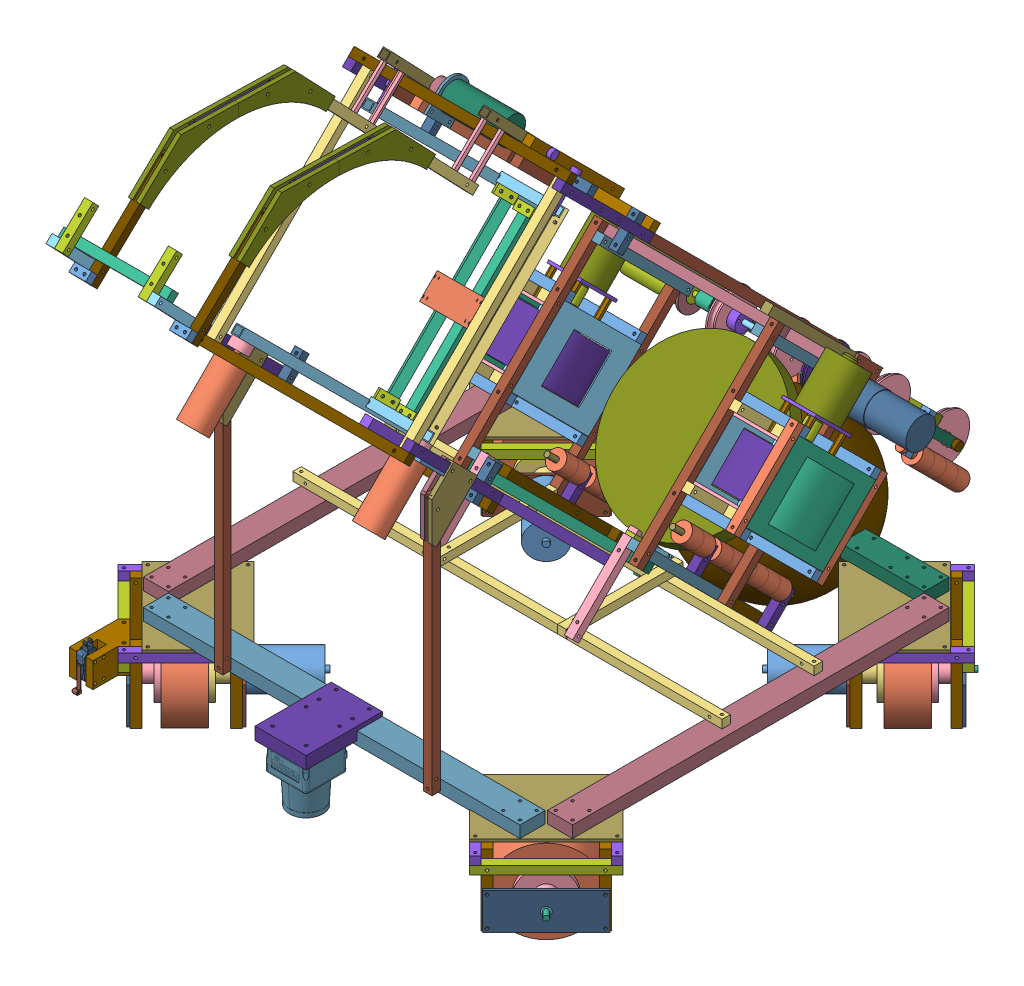
SolidWorks assembly R2, configuration ﾃﾞﾌｫﾙﾄ. Lengths in mm. (continued)
Components (placement in the parent): (continued)
- Copy of Shooter^R2-1: Copy of Shooter^R2 [ﾃﾞﾌｫﾙﾄ] at (-133.6019 -3.3981 619.3345) x (1 0 0) z (0 0.707107 0.707107) size (512.8 347.34 409.41) (virtual, flexible) (continued)
  - Copy of Copy of Copy (2) of Copy of Copy (2) of Copy of Copy (2) of 角材１^Copy of Shooter_R2-3: Copy of Copy of Copy (2) of Copy of Copy (2) of Copy of Copy (2) of 角材１^Copy of Shooter_R2 [ﾃﾞﾌｫﾙﾄ] at (20 10 0) x (0 0 1) z (-1 0 0) size (150 10 10) (virtual)
  - Copy of Copy of Copy (2) of Copy of Copy (2) of Copy of Copy (2) of 角材１^Copy of Shooter_R2-4: Copy of Copy of Copy (2) of Copy of Copy (2) of Copy of Copy (2) of 角材１^Copy of Shooter_R2 [ﾃﾞﾌｫﾙﾄ] at (210 10 0) x (0 0 1) z (-1 0 0) size (150 10 10) (virtual)
  - Part19^Copy of Shooter_R2-1: Part19^Copy of Shooter_R2 [ﾃﾞﾌｫﾙﾄ] at (290 165 10) x (-1 0 0) z (0 0 -1) size (190 190 20) (virtual)
  - Copy (2) of Copy of Copy of Copy of Copy of Copy (2) of Copy of Copy (2) of 角材１^Copy of Shooter_R2-3: Copy (2) of Copy of Copy of Copy of Copy of Copy (2) of Copy of Copy (2) of 角材１^Copy of Shooter_R2 [ﾃﾞﾌｫﾙﾄ] at (180 50 20) x (0 -1 0) z (0 0 1) size (50 10 10) (virtual)
  - Copy of Copy (2) of Copy of Copy of Copy of Copy of Copy (2) of Copy of Copy (2) of 角材１^Copy of Shooter_R2-1: Copy of Copy (2) of Copy of Copy of Copy of Copy of Copy (2) of Copy of Copy (2) of 角材１^Copy of Shooter_R2 [ﾃﾞﾌｫﾙﾄ] at (170 10 140) x (0 0 -1) z (1 0 0) size (250 10 10) (virtual)
  - Part17^Copy of Shooter_R2-2: Part17^Copy of Shooter_R2 [ﾃﾞﾌｫﾙﾄ] at (35 45 -115) x (-0.307741 0.95147 0) z (0 0 1) size (6 6 200) (virtual)
  - Copy (2) of Copy of Copy of Copy of Copy of Copy (2) of Copy of Copy (2) of 角材１^Copy of Shooter_R2-5: Copy (2) of Copy of Copy of Copy of Copy of Copy (2) of Copy of Copy (2) of 角材１^Copy of Shooter_R2 [ﾃﾞﾌｫﾙﾄ] at (30 50 20) x (0 -1 0) z (0 0 1) size (50 10 10) (virtual)
  - Copy of Copy (2) of Copy of Copy of Copy of Copy of Copy (2) of Copy of Copy (2) of 角材１^Copy of Shooter_R2-2: Copy of Copy (2) of Copy of Copy of Copy of Copy of Copy (2) of Copy of Copy (2) of 角材１^Copy of Shooter_R2 [ﾃﾞﾌｫﾙﾄ] at (40 10 140) x (0 0 -1) z (1 0 0) size (250 10 10) (virtual)
  - Copy (3) of Copy of Copy of Copy of Copy of Copy (2) of Copy of Copy (2) of 角材１^Copy of Shooter_R2-1: Copy (3) of Copy of Copy of Copy of Copy of Copy (2) of Copy of Copy (2) of 角材１^Copy of Shooter_R2 [ﾃﾞﾌｫﾙﾄ] at (30 0 -100) size (160 10 10) (virtual)
  - Copy (2) of Copy of Copy of Copy of Copy of Copy (2) of Copy of Copy (2) of 角材１^Copy of Shooter_R2-6: Copy (2) of Copy of Copy of Copy of Copy of Copy (2) of Copy of Copy (2) of 角材１^Copy of Shooter_R2 [ﾃﾞﾌｫﾙﾄ] at (30 50 -110) x (0 -1 0) z (0 0 1) size (50 10 10) (virtual)
  - Copy (2) of Copy of Copy of Copy of Copy of Copy (2) of Copy of Copy (2) of 角材１^Copy of Shooter_R2-7: Copy (2) of Copy of Copy of Copy of Copy of Copy (2) of Copy of Copy (2) of 角材１^Copy of Shooter_R2 [ﾃﾞﾌｫﾙﾄ] at (180 50 -110) x (0 -1 0) z (0 0 1) size (50 10 10) (virtual)
  - Part20^Copy of Shooter_R2-1: Part20^Copy of Shooter_R2 [ﾃﾞﾌｫﾙﾄ] at (185 45 0.2) x (0 1 0) z (0 0 -1) size (21 21 19.8) (virtual)
  - Part20^Copy of Shooter_R2-2: Part20^Copy of Shooter_R2 [ﾃﾞﾌｫﾙﾄ] at (185 45 20) x (0 1 0) z (0 0 -1) size (21 21 19.8) (virtual)
  - Part20^Copy of Shooter_R2-3: Part20^Copy of Shooter_R2 [ﾃﾞﾌｫﾙﾄ] at (185 45 -79) x (0 1 0) z (0 0 -1) size (21 21 19.8) (virtual)
  - Part20^Copy of Shooter_R2-4: Part20^Copy of Shooter_R2 [ﾃﾞﾌｫﾙﾄ] at (185 45 -19.6) x (0 1 0) z (0 0 -1) size (21 21 19.8) (virtual)
  - Part20^Copy of Shooter_R2-5: Part20^Copy of Shooter_R2 [ﾃﾞﾌｫﾙﾄ] at (185 45 -59.2) x (0 1 0) z (0 0 -1) size (21 21 19.8) (virtual)
  - Part20^Copy of Shooter_R2-6: Part20^Copy of Shooter_R2 [ﾃﾞﾌｫﾙﾄ] at (185 45 -39.4) x (0.985931 0.167151 0) z (0 0 -1) size (21 21 19.8) (virtual)
  - Part20^Copy of Shooter_R2-7: Part20^Copy of Shooter_R2 [ﾃﾞﾌｫﾙﾄ] at (35 45 -19.6) x (0 1 0) z (0 0 -1) size (21 21 19.8) (virtual)
  - Part20^Copy of Shooter_R2-8: Part20^Copy of Shooter_R2 [ﾃﾞﾌｫﾙﾄ] at (35 45 20) x (0 1 0) z (0 0 -1) size (21 21 19.8) (virtual)
  - Part20^Copy of Shooter_R2-9: Part20^Copy of Shooter_R2 [ﾃﾞﾌｫﾙﾄ] at (35 45 -39.4) x (0 1 0) z (0 0 -1) size (21 21 19.8) (virtual)
  - Part20^Copy of Shooter_R2-10: Part20^Copy of Shooter_R2 [ﾃﾞﾌｫﾙﾄ] at (35 45 0.2) x (0 1 0) z (0 0 -1) size (21 21 19.8) (virtual)
  - Part20^Copy of Shooter_R2-11: Part20^Copy of Shooter_R2 [ﾃﾞﾌｫﾙﾄ] at (35 45 -59.2) x (0.234145 0.972202 0) z (0 0 -1) size (21 21 19.8) (virtual)
  - Part20^Copy of Shooter_R2-12: Part20^Copy of Shooter_R2 [ﾃﾞﾌｫﾙﾄ] at (35 45 -79) x (0 1 0) z (0 0 -1) size (21 21 19.8) (virtual)
  - Part20^Copy of Shooter_R2-21: Part20^Copy of Shooter_R2 [ﾃﾞﾌｫﾙﾄ] at (35 45 69.6) x (0 1 0) z (0 0 -1) size (21 21 19.8) (virtual)
  - Part20^Copy of Shooter_R2-22: Part20^Copy of Shooter_R2 [ﾃﾞﾌｫﾙﾄ] at (35 45 49.8) x (0 1 0) z (0 0 -1) size (21 21 19.8) (virtual)
  - Part20^Copy of Shooter_R2-23: Part20^Copy of Shooter_R2 [ﾃﾞﾌｫﾙﾄ] at (185 45 69.6) x (0.413014 0.910725 0) z (0 0 -1) size (21 21 19.8) (virtual)
  - Part20^Copy of Shooter_R2-24: Part20^Copy of Shooter_R2 [ﾃﾞﾌｫﾙﾄ] at (185 45 49.8) x (-0.320274 0.947325 0) z (0 0 -1) size (21 21 19.8) (virtual)
  - Copy of Copy of Copy of Copy (2) of Copy of Copy (2) of Copy of Copy (2) of 角材１^Copy of Shooter_R2-1: Copy of Copy of Copy of Copy (2) of Copy of Copy (2) of Copy of Copy (2) of 角材１^Copy of Shooter_R2 [ﾃﾞﾌｫﾙﾄ] at (190 16.9239 46.0051) x (0 -0.707107 0.707107) z (-1 0 0) size (140 10 10) (virtual)
  - Copy of Copy of Copy of Copy (2) of Copy of Copy (2) of Copy of Copy (2) of 角材１^Copy of Shooter_R2-2: Copy of Copy of Copy of Copy (2) of Copy of Copy (2) of Copy of Copy (2) of 角材１^Copy of Shooter_R2 [ﾃﾞﾌｫﾙﾄ] at (40 16.9239 46.0051) x (0 -0.707107 0.707107) z (-1 0 0) size (140 10 10) (virtual)
  - Copy (2) of Copy of Copy of Copy of Copy (2) of Copy of Copy (2) of 角材１^Copy of Shooter_R2-1: Copy (2) of Copy of Copy of Copy of Copy (2) of Copy of Copy (2) of 角材１^Copy of Shooter_R2 [ﾃﾞﾌｫﾙﾄ] at (190 20 150) x (0 -1 0) z (1 0 0) size (100 10 10) (virtual)
  - Copy (2) of Copy of Copy of Copy of Copy (2) of Copy of Copy (2) of 角材１^Copy of Shooter_R2-2: Copy (2) of Copy of Copy of Copy of Copy (2) of Copy of Copy (2) of 角材１^Copy of Shooter_R2 [ﾃﾞﾌｫﾙﾄ] at (20 20 150) x (0 -1 0) z (1 0 0) size (100 10 10) (virtual)
  - Copy of Part14^Copy of Shooter_R2-1: Copy of Part14^Copy of Shooter_R2 [ﾃﾞﾌｫﾙﾄ] at (45.3993 224.2591 -11.1142) x (0 0.083089 -0.996542) z (0 -0.996542 -0.083089) size (6 150 6) (virtual)
  - Copy of Copy of Copy of Copy (2) of Part36^Copy of Shooter_R2-1: Copy of Copy of Copy of Copy (2) of Part36^Copy of Shooter_R2 [ﾃﾞﾌｫﾙﾄ] at (36.0219 185.9032 -80.4602) x (0 0.839725 -0.543011) z (-1 0 0) size (16 16 18) (virtual)
  - Copy (2) of Copy of Part33^Copy of Shooter_R2-2: Copy (2) of Copy of Part33^Copy of Shooter_R2 [ﾃﾞﾌｫﾙﾄ] at (-597.1629 304.0265 -20) x (1 0 0) z (0 0 -1) size (90 32 32) (virtual)
  - Copy (2) of Copy (2) of Part36^Copy of Shooter_R2-2: Copy (2) of Copy (2) of Part36^Copy of Shooter_R2 [ﾃﾞﾌｫﾙﾄ] at (151 153.9641 -31.7433) x (0 -0.163101 0.986609) z (1 0 0) size (22 22 10) (virtual)
  - Copy of Copy of Part36^Copy of Shooter_R2-1: Copy of Copy of Part36^Copy of Shooter_R2 [ﾃﾞﾌｫﾙﾄ] at (179.9858 153.1375 -24.4469) x (0 -0.061762 0.998091) z (1 0 0) size (22 22 10) (virtual)
  - Part22^Copy of Shooter_R2-1: Part22^Copy of Shooter_R2 [ﾃﾞﾌｫﾙﾄ] at (285 218 -20) x (0 0 1) z (0 -1 0) size (37 103 37) (virtual)
  - Part23^Copy of Shooter_R2-1: Part23^Copy of Shooter_R2 [ﾃﾞﾌｫﾙﾄ] at (203 240 -40) x (0 0 1) z (-1 0 0) size (40 52 3) (virtual)
  - Copy of Copy of Copy (2) of Copy of Copy of Copy of Copy of Copy (2) of Copy of Copy (2) of 角材１^Copy of Shooter_R2-1: Copy of Copy of Copy (2) of Copy of Copy of Copy of Copy of Copy (2) of Copy of Copy (2) of 角材１^Copy of Shooter_R2 [ﾃﾞﾌｫﾙﾄ] at (190 240 140) x (0 0 -1) z (1 0 0) size (180 10 10) (virtual)
  - Copy of Copy of Copy (2) of Copy of Copy of Copy of Copy of Copy (2) of Copy of Copy (2) of 角材１^Copy of Shooter_R2-2: Copy of Copy of Copy (2) of Copy of Copy of Copy of Copy of Copy (2) of Copy of Copy (2) of 角材１^Copy of Shooter_R2 [ﾃﾞﾌｫﾙﾄ] at (20 240 140) x (0 0 -1) z (1 0 0) size (180 10 10) (virtual)
  - Part24^Copy of Shooter_R2-1: Part24^Copy of Shooter_R2 [ﾃﾞﾌｫﾙﾄ] at (7 250 -40) x (0 0 1) z (1 0 0) size (40 45 3) (virtual)
  - Copy (4) of Copy of Copy of Copy of Copy of Copy (2) of Copy of Copy (2) of 角材１^Copy of Shooter_R2-2: Copy (4) of Copy of Copy of Copy of Copy of Copy (2) of Copy of Copy (2) of 角材１^Copy of Shooter_R2 [ﾃﾞﾌｫﾙﾄ] at (0 0 10) size (220 10 10) (virtual)
  - Copy (2) of Copy of Copy of Copy of Copy of Copy of Copy of Copy of Copy (2) of Copy of Copy (9) of Copy (2) of 角材１^Copy of Shooter_R2-3: Copy (2) of Copy of Copy of Copy of Copy of Copy of Copy of Copy of Copy (2) of Copy of Copy (9) of Copy (2) of 角材１^Copy of Shooter_R2 [ﾃﾞﾌｫﾙﾄ] at (50 230 -5) x (0 0 -1) z (-1 0 0) size (220 10 10) (virtual)
  - Copy (2) of Copy of Copy of Copy of Copy of Copy of Copy of Copy of Copy (2) of Copy of Copy (9) of Copy (2) of 角材１^Copy of Shooter_R2-4: Copy (2) of Copy of Copy of Copy of Copy of Copy of Copy of Copy of Copy (2) of Copy of Copy (9) of Copy (2) of 角材１^Copy of Shooter_R2 [ﾃﾞﾌｫﾙﾄ] at (180 230 -5) x (0 0 -1) z (-1 0 0) size (220 10 10) (virtual)
  - Copy of Copy of Copy of Copy (2) of Copy of Copy (2) of 角材１^Copy of Shooter_R2-1: Copy of Copy of Copy of Copy (2) of Copy of Copy (2) of 角材１^Copy of Shooter_R2 [ﾃﾞﾌｫﾙﾄ] at (190 240 -170) x (-1 0 0) z (0 0 1) size (160 10 10) (virtual)
  - Copy of Part25^Copy of Shooter_R2-7: Copy of Part25^Copy of Shooter_R2 [ﾃﾞﾌｫﾙﾄ] at (169 225 -20) x (1 0 0) z (0 0.163101 -0.986609) size (8 56 56) (virtual)
  - Copy (2) of Copy (2) of Part36^Copy of Shooter_R2-3: Copy (2) of Copy (2) of Part36^Copy of Shooter_R2 [ﾃﾞﾌｫﾙﾄ] at (69 295.1733 -3.8846) x (0 -0.223824 0.974629) z (-1 0 0) size (22 22 10) (virtual)
  - Part26^Copy of Shooter_R2-3: Part26^Copy of Shooter_R2 [ﾃﾞﾌｫﾙﾄ] at (185 225 -220) x (-1 0 0) z (0 0.743251 -0.669013) size (35 10 10) (virtual)
  - Part26^Copy of Shooter_R2-4: Part26^Copy of Shooter_R2 [ﾃﾞﾌｫﾙﾄ] at (35 225 -220) x (1 0 0) z (0 -0.001736 -0.999998) size (35 10 10) (virtual)
  - Part26^Copy of Shooter_R2-5: Part26^Copy of Shooter_R2 [ﾃﾞﾌｫﾙﾄ] at (185 225 -120) x (-1 0 0) z (0 -0.001736 -0.999998) size (35 10 10) (virtual)
  - Part26^Copy of Shooter_R2-6: Part26^Copy of Shooter_R2 [ﾃﾞﾌｫﾙﾄ] at (35 225 -120) x (1 0 0) z (0 -0.001736 -0.999998) size (35 10 10) (virtual)
  - Copy (3) of Copy of Copy of Copy of Copy (2) of Copy of Copy (2) of 角材１^Copy of Shooter_R2-1: Copy (3) of Copy of Copy of Copy of Copy (2) of Copy of Copy (2) of 角材１^Copy of Shooter_R2 [ﾃﾞﾌｫﾙﾄ] at (190 195 -160) x (0 1 0) z (0 0 1) size (45 10 10) (virtual)
  - Copy (3) of Copy of Copy of Copy of Copy (2) of Copy of Copy (2) of 角材１^Copy of Shooter_R2-2: Copy (3) of Copy of Copy of Copy of Copy (2) of Copy of Copy (2) of 角材１^Copy of Shooter_R2 [ﾃﾞﾌｫﾙﾄ] at (40 195 -160) x (0 1 0) z (0 0 1) size (45 10 10) (virtual)
  - Part20^Copy of Shooter_R2-25: Part20^Copy of Shooter_R2 [ﾃﾞﾌｫﾙﾄ] at (185 200 -184.8) x (0.035115 -0.999383 0) z (0 0 1) size (21 21 19.8) (virtual)
  - Copy of Part26^Copy of Shooter_R2-1: Copy of Part26^Copy of Shooter_R2 [ﾃﾞﾌｫﾙﾄ] at (185 200 -145) x (0 0 -1) z (-0.990327 0.138756 0) size (105 10 10) (virtual)
  - Part20^Copy of Shooter_R2-26: Part20^Copy of Shooter_R2 [ﾃﾞﾌｫﾙﾄ] at (185 200 -204.6) x (-0.121292 -0.992617 0) z (0 0 1) size (21 21 19.8) (virtual)
  - Part20^Copy of Shooter_R2-27: Part20^Copy of Shooter_R2 [ﾃﾞﾌｫﾙﾄ] at (185 200 -224.4) x (0.035115 -0.999383 0) z (0 0 1) size (21 21 19.8) (virtual)
  - Part20^Copy of Shooter_R2-28: Part20^Copy of Shooter_R2 [ﾃﾞﾌｫﾙﾄ] at (185 200 -244.2) x (0.035115 -0.999383 0) z (0 0 1) size (21 21 19.8) (virtual)
  - Part20^Copy of Shooter_R2-29: Part20^Copy of Shooter_R2 [ﾃﾞﾌｫﾙﾄ] at (35 200 -184.8) x (0.035115 -0.999383 0) z (0 0 1) size (21 21 19.8) (virtual)
  - Part20^Copy of Shooter_R2-30: Part20^Copy of Shooter_R2 [ﾃﾞﾌｫﾙﾄ] at (35 200 -204.6) x (-0.121292 -0.992617 0) z (0 0 1) size (21 21 19.8) (virtual)
  - Copy of Part26^Copy of Shooter_R2-2: Copy of Part26^Copy of Shooter_R2 [ﾃﾞﾌｫﾙﾄ] at (35 200 -145) x (0 0 -1) z (-0.990327 0.138756 0) size (105 10 10) (virtual)
  - Part20^Copy of Shooter_R2-31: Part20^Copy of Shooter_R2 [ﾃﾞﾌｫﾙﾄ] at (35 200 -224.4) x (0.035115 -0.999383 0) z (0 0 1) size (21 21 19.8) (virtual)
  - Part20^Copy of Shooter_R2-32: Part20^Copy of Shooter_R2 [ﾃﾞﾌｫﾙﾄ] at (35 200 -244.2) x (0.035115 -0.999383 0) z (0 0 1) size (21 21 19.8) (virtual)
  - Copy of Copy (4) of Copy of Copy of Copy of Copy (2) of Copy of Copy (2) of 角材１^Copy of Shooter_R2-1: Copy of Copy (4) of Copy of Copy of Copy of Copy (2) of Copy of Copy (2) of 角材１^Copy of Shooter_R2 [ﾃﾞﾌｫﾙﾄ] at (366.4 -75 137.9289) x (-1 0 0) z (0 -0.707107 -0.707107) size (512.8 10 10) (virtual)
  - Copy of Copy (4) of Copy of Copy of Copy of Copy (2) of Copy of Copy (2) of 角材１^Copy of Shooter_R2-2: Copy of Copy (4) of Copy of Copy of Copy of Copy (2) of Copy of Copy (2) of 角材１^Copy of Shooter_R2 [ﾃﾞﾌｫﾙﾄ] at (366.4 2.7817 60.1472) x (-1 0 0) z (0 -0.707107 -0.707107) size (512.8 10 10) (virtual)
  - Part25^Copy of Shooter_R2-5: Part25^Copy of Shooter_R2 [ﾃﾞﾌｫﾙﾄ] at (169 225 -120) x (1 0 0) z (0 -0.163101 0.986609) size (8 56 56) (virtual)
  - Part25^Copy of Shooter_R2-6: Part25^Copy of Shooter_R2 [ﾃﾞﾌｫﾙﾄ] at (169 225 -220) x (1 0 0) z (0 0.431687 0.902023) size (8 56 56) (virtual)
  - Part25^Copy of Shooter_R2-7: Part25^Copy of Shooter_R2 [ﾃﾞﾌｫﾙﾄ] at (51 225 -120) x (-1 0 0) z (0 -0.974129 -0.225994) size (8 56 56) (virtual)
  - Part25^Copy of Shooter_R2-8: Part25^Copy of Shooter_R2 [ﾃﾞﾌｫﾙﾄ] at (51 225 -220) x (-1 0 0) z (0 -0.974129 -0.225994) size (8 56 56) (virtual)
  - Part27^Copy of Shooter_R2-1: Part27^Copy of Shooter_R2 [ﾃﾞﾌｫﾙﾄ] at (0 155.2 149.8) x (0 0 -1) z (1 0 0) size (129.6 89.6 10) (virtual)
  - Copy of Part27^Copy of Shooter_R2-1: Copy of Part27^Copy of Shooter_R2 [ﾃﾞﾌｫﾙﾄ] at (280 155.2 149.8) x (0 0 -1) z (1 0 0) size (129.6 89.6 26) (virtual)
  - Part27^Copy of Shooter_R2-3: Part27^Copy of Shooter_R2 [ﾃﾞﾌｫﾙﾄ] at (220 154.8 -0.2) x (0 0 1) z (-1 0 0) size (129.6 89.6 10) (virtual)
  - Copy of Part27^Copy of Shooter_R2-2: Copy of Part27^Copy of Shooter_R2 [ﾃﾞﾌｫﾙﾄ] at (-60 155.2 -0.2) x (0 0 1) z (-1 0 0) size (129.6 89.6 26) (virtual)
  - Copy of Copy of Part9^Copy of Shooter_R2-1: Copy of Copy of Part9^Copy of Shooter_R2 [ﾃﾞﾌｫﾙﾄ] at (115.15 -0.5946 0.9681) x (0 0 1) z (-1 0 0) size (50 10.5 10) (virtual)
  - Copy of Copy of Part8^Copy of Shooter_R2-1: Copy of Copy of Part8^Copy of Shooter_R2 [ﾃﾞﾌｫﾙﾄ] at (125.15 -0.5946 0.9681) x (0 0 1) z (-1 0 0) size (42.8 26.9 30.3) (virtual)
  - Copy of Copy of D3V-016-1C23^Copy of Shooter_R2-1: Copy of Copy of D3V-016-1C23^Copy of Shooter_R2 [ﾃﾞﾌｫﾙﾄ] at (105.15 -0.25 2.2) x (-1 0 0) z (0 0 -1) size (10.3 26.4 49.2) (virtual)
    - D3V_016_1C23_BASE^Copy of Copy of D3V-016-1C23_Copy of Shooter_R2-1: D3V_016_1C23_BASE^Copy of Copy of D3V-016-1C23_Copy of Shooter_R2 [ﾃﾞﾌｫﾙﾄ] at origin size (10.3 19.05 37.8) (virtual)
    - D3V_016_1C23_LEVER^Copy of Copy of D3V-016-1C23_Copy of Shooter_R2-1: D3V_016_1C23_LEVER^Copy of Copy of D3V-016-1C23_Copy of Shooter_R2 [ﾃﾞﾌｫﾙﾄ] at (-4.8 14.7 -11.8) x (0 0 -1) z (1 0 0) size (28.3 7.35 7.1) (virtual)
    - D3V_016_1C23_BUTTON^Copy of Copy of D3V-016-1C23_Copy of Shooter_R2-1: D3V_016_1C23_BUTTON^Copy of Copy of D3V-016-1C23_Copy of Shooter_R2 [ﾃﾞﾌｫﾙﾄ] at (-4.85 11.6 2) size (4.3 3.1 2.8) (virtual)
  - Copy of Copy (2) of Copy of Part9^Copy of Shooter_R2-1: Copy of Copy (2) of Copy of Part9^Copy of Shooter_R2 [ﾃﾞﾌｫﾙﾄ] at (104.85 240.3946 -179.0319) x (0 0 1) z (1 0 0) size (100 13.5 10) (virtual)
  - Copy (2) of Copy of Part8^Copy of Shooter_R2-2: Copy (2) of Copy of Part8^Copy of Shooter_R2 [ﾃﾞﾌｫﾙﾄ] at (94.85 240.3946 -179.0319) x (0 0 1) z (1 0 0) size (42.8 26.9 30.3) (virtual)
  - Copy (2) of Copy of D3V-016-1C23^Copy of Shooter_R2-2: Copy (2) of Copy of D3V-016-1C23^Copy of Shooter_R2 [ﾃﾞﾌｫﾙﾄ] at (114.85 240.05 -177.8) x (1 0 0) z (0 0 -1) size (10.3 26.4 49.2) (virtual)
    - D3V_016_1C23_BASE^Copy (2) of Copy of D3V-016-1C23_Copy of Shooter_R2-1: D3V_016_1C23_BASE^Copy (2) of Copy of D3V-016-1C23_Copy of Shooter_R2 [ﾃﾞﾌｫﾙﾄ] at origin size (10.3 19.05 37.8) (virtual)
    - D3V_016_1C23_LEVER^Copy (2) of Copy of D3V-016-1C23_Copy of Shooter_R2-1: D3V_016_1C23_LEVER^Copy (2) of Copy of D3V-016-1C23_Copy of Shooter_R2 [ﾃﾞﾌｫﾙﾄ] at (-4.8 14.7 -11.8) x (0 0 -1) z (1 0 0) size (28.3 7.35 7.1) (virtual)
    - D3V_016_1C23_BUTTON^Copy (2) of Copy of D3V-016-1C23_Copy of Shooter_R2-1: D3V_016_1C23_BUTTON^Copy (2) of Copy of D3V-016-1C23_Copy of Shooter_R2 [ﾃﾞﾌｫﾙﾄ] at (-4.85 11.6 2) size (4.3 3.1 2.8) (virtual)
  - Part25^Copy of Shooter_R2-9: Part25^Copy of Shooter_R2 [ﾃﾞﾌｫﾙﾄ] at (51 225 -20) x (-1 0 0) z (0 -0.974129 -0.225994) size (8 56 56) (virtual)
- Copy of Rail^R2-1: Copy of Rail^R2 [ﾃﾞﾌｫﾙﾄ] at (-153.6019 377.0254 1016.7285) x (1 0 0) z (0 0.707107 0.707107) size (260 373 863.92) (virtual, flexible)
  - Copy of 角材１^Copy of Rail_R2-1: Copy of 角材１^Copy of Rail_R2 [ﾃﾞﾌｫﾙﾄ] at (260 10 -150) x (0 0 1) z (0 -1 0) size (150 10 10) (virtual)
  - Copy of 角材１^Copy of Rail_R2-2: Copy of 角材１^Copy of Rail_R2 [ﾃﾞﾌｫﾙﾄ] at (10 10 -150) x (0 0 1) z (0 -1 0) size (150 10 10) (virtual)
  - Copy of Copy of 角材１^Copy of Rail_R2-1: Copy of Copy of 角材１^Copy of Rail_R2 [ﾃﾞﾌｫﾙﾄ] at (0 0 -10) x (1 0 0) z (0 -1 0) size (260 10 10) (virtual)
  - Copy of Part24^Copy of Rail_R2-1: Copy of Part24^Copy of Rail_R2 [ﾃﾞﾌｫﾙﾄ] at (260 -3 -20) x (0 0 -1) z (0 1 0) size (40 45 3) (virtual)
  - Copy of Copy (2) of Copy of Part33^Copy of Rail_R2-1: Copy of Copy (2) of Copy of Part33^Copy of Rail_R2 [ﾃﾞﾌｫﾙﾄ] at (314.0265 -607.1629 -40) x (0 1 0) z (0 0 1) size (90 32 32) (virtual)
  - Copy of Copy of Copy of 角材１^Copy of Rail_R2-1: Copy of Copy of Copy of 角材１^Copy of Rail_R2 [ﾃﾞﾌｫﾙﾄ] at (240 -10 -10) x (0 1 0) z (0 0 -1) size (284 10 10) (virtual)
  - Copy of Copy of Copy of 角材１^Copy of Rail_R2-2: Copy of Copy of Copy of 角材１^Copy of Rail_R2 [ﾃﾞﾌｫﾙﾄ] at (10 -10 -10) x (0 1 0) z (0 0 -1) size (284 10 10) (virtual)
  - Copy of Copy of Copy of Part36^Copy of Rail_R2-1: Copy of Copy of Copy of Part36^Copy of Rail_R2 [ﾃﾞﾌｫﾙﾄ] at (285.6516 15 -91.1704) x (-0.7107 0 -0.703495) z (0 -1 0) size (22 22 10) (virtual)
  - Copy of Copy (2) of Copy of Copy of Copy of Copy of Copy of Copy of Copy of Copy (2) of Copy of Copy (9) of Copy (2) of 角材１^Copy of Rail_R2-1: Copy of Copy (2) of Copy of Copy of Copy of Copy of Copy of Copy of Copy of Copy (2) of Copy of Copy (9) of Copy (2) of 角材１^Copy of Rail_R2 [ﾃﾞﾌｫﾙﾄ] at (249.178 15 -33.0011) x (-0.7107 0 -0.703495) z (0 1 0) size (300 10 10) (virtual)
  - Copy of Copy of Copy of Copy of 角材１^Copy of Rail_R2-1: Copy of Copy of Copy of Copy of 角材１^Copy of Rail_R2 [ﾃﾞﾌｫﾙﾄ] at (35.9679 15 -244.0495) x (0 1 0) z (0.703495 0 -0.7107) size (230 10 10) (virtual)
  - Copy of Copy of Copy of Copy of Copy of 角材１^Copy of Rail_R2-1: Copy of Copy of Copy of Copy of Copy of 角材１^Copy of Rail_R2 [ﾃﾞﾌｫﾙﾄ] at (36.0399 35 -229.9076) x (0.703495 0 -0.7107) z (0 -1 0) size (20 10 10) (virtual)
  - Copy of Copy of Copy of Copy of Copy of 角材１^Copy of Rail_R2-2: Copy of Copy of Copy of Copy of Copy of 角材１^Copy of Rail_R2 [ﾃﾞﾌｫﾙﾄ] at (36.0399 235 -229.9076) x (0.703495 0 -0.7107) z (0 -1 0) size (20 10 10) (virtual)
  - Copy of Copy (2) of Copy of Copy of Copy of Copy of Copy of Copy of Copy of Copy (2) of Copy of Copy (9) of Copy (2) of 角材１^Copy of Rail_R2-2: Copy of Copy (2) of Copy of Copy of Copy of Copy of Copy of Copy of Copy of Copy (2) of Copy of Copy (9) of Copy (2) of 角材１^Copy of Rail_R2 [ﾃﾞﾌｫﾙﾄ] at (249.178 235 -33.0011) x (-0.7107 0 -0.703495) z (0 1 0) size (300 10 10) (virtual)
  - Copy of Copy of Copy of Copy of Copy of 角材１^Copy of Rail_R2-3: Copy of Copy of Copy of Copy of Copy of 角材１^Copy of Rail_R2 [ﾃﾞﾌｫﾙﾄ] at (29.985 22 -315.0003) x (-1 0 0.000054) z (0 1 0) size (20 10 10) (virtual)
  - Copy of Copy of Copy of Copy of Copy of 角材１^Copy of Rail_R2-4: Copy of Copy of Copy of Copy of Copy of 角材１^Copy of Rail_R2 [ﾃﾞﾌｫﾙﾄ] at (29.985 222 -315.0003) x (-1 0 0.000054) z (0 1 0) size (20 10 10) (virtual)
  - Copy of Copy (2) of Copy of Copy of Copy of Copy of Copy of Copy of Copy of Copy (2) of Copy of Copy (9) of Copy (2) of 角材１^Copy of Rail_R2-3: Copy of Copy (2) of Copy of Copy of Copy of Copy of Copy of Copy of Copy of Copy (2) of Copy of Copy (9) of Copy (2) of 角材１^Copy of Rail_R2 [ﾃﾞﾌｫﾙﾄ] at (20.0008 22 -24.9997) x (-0.000054 0 -1) z (0 -1 0) size (300 10 10) (virtual)
  - Copy of Copy (2) of Copy of Copy of Copy of Copy of Copy of Copy of Copy of Copy (2) of Copy of Copy (9) of Copy (2) of 角材１^Copy of Rail_R2-4: Copy of Copy (2) of Copy of Copy of Copy of Copy of Copy of Copy of Copy of Copy (2) of Copy of Copy (9) of Copy (2) of 角材１^Copy of Rail_R2 [ﾃﾞﾌｫﾙﾄ] at (20.0008 242 -24.9997) x (-0.000054 0 -1) z (0 -1 0) size (300 10 10) (virtual)
  - Copy of Copy of Copy of Copy of 角材１^Copy of Rail_R2-3: Copy of Copy of Copy of Copy of 角材１^Copy of Rail_R2 [ﾃﾞﾌｫﾙﾄ] at (19.9845 242 -324.9997) x (0 -1 0) z (-1 0 0.000054) size (230 10 10) (virtual)
  - Copy of Copy (2) of Copy of Part33^Copy of Rail_R2-2: Copy of Copy (2) of Copy of Part33^Copy of Rail_R2 [ﾃﾞﾌｫﾙﾄ] at (-54.0265 -607.1629 -40) x (0 1 0) z (0 0 -1) size (90 32 32) (virtual)
  - Copy of Part24^Copy of Rail_R2-2: Copy of Part24^Copy of Rail_R2 [ﾃﾞﾌｫﾙﾄ] at (0 -3 -60) x (0 0 1) z (0 1 0) size (40 45 3) (virtual)
  - Copy of Copy of Copy of Part36^Copy of Rail_R2-2: Copy of Copy of Copy of Part36^Copy of Rail_R2 [ﾃﾞﾌｫﾙﾄ] at (-47 12 -39.9961) x (0.000054 0 1) z (0 -1 0) size (22 22 10) (virtual)
  - Copy (2) of Copy (2) of Copy of Copy of Copy of Copy of 角材１^Copy of Rail_R2-1: Copy (2) of Copy (2) of Copy of Copy of Copy of Copy of 角材１^Copy of Rail_R2 [ﾃﾞﾌｫﾙﾄ] at (210 10 -420) x (0 0 1) z (0 -1 0) size (420 10 10) (virtual)
  - Copy of Copy of 角材１^Copy of Rail_R2-3: Copy of Copy of 角材１^Copy of Rail_R2 [ﾃﾞﾌｫﾙﾄ] at (0 0 -150) x (1 0 0) z (0 -1 0) size (260 10 10) (virtual)
  - Copy of 角材１^Copy of Rail_R2-5: Copy of 角材１^Copy of Rail_R2 [ﾃﾞﾌｫﾙﾄ] at (0 254 -150) x (0 0 1) z (0 1 0) size (150 10 10) (virtual)
  - Copy of Copy of 角材１^Copy of Rail_R2-4: Copy of Copy of 角材１^Copy of Rail_R2 [ﾃﾞﾌｫﾙﾄ] at (260 264 -10) x (-1 0 0) z (0 1 0) size (260 10 10) (virtual)
  - Copy of 角材１^Copy of Rail_R2-6: Copy of 角材１^Copy of Rail_R2 [ﾃﾞﾌｫﾙﾄ] at (250 254 -150) x (0 0 1) z (0 1 0) size (150 10 10) (virtual)
  - Copy (2) of Copy of Copy of 角材１^Copy of Rail_R2-1: Copy (2) of Copy of Copy of 角材１^Copy of Rail_R2 [ﾃﾞﾌｫﾙﾄ] at (260 264 -150) x (-1 0 0) z (0 1 0) size (260 10 10) (virtual)
  - Copy (2) of Copy of Copy of Copy of 角材１^Copy of Rail_R2-1: Copy (2) of Copy of Copy of Copy of 角材１^Copy of Rail_R2 [ﾃﾞﾌｫﾙﾄ] at (10 -10 -130) x (0 1 0) z (0 0 -1) size (40 10 10) (virtual)
  - Copy (2) of Copy of Copy of Copy of 角材１^Copy of Rail_R2-2: Copy (2) of Copy of Copy of Copy of 角材１^Copy of Rail_R2 [ﾃﾞﾌｫﾙﾄ] at (240 -10 -130) x (0 1 0) z (0 0 -1) size (40 10 10) (virtual)
  - Copy (2) of Copy of Copy of Copy of 角材１^Copy of Rail_R2-3: Copy (2) of Copy of Copy of Copy of 角材１^Copy of Rail_R2 [ﾃﾞﾌｫﾙﾄ] at (240 234 -130) x (0 1 0) z (0 0 -1) size (40 10 10) (virtual)
  - Copy (2) of Copy of Copy of Copy of 角材１^Copy of Rail_R2-4: Copy (2) of Copy of Copy of Copy of 角材１^Copy of Rail_R2 [ﾃﾞﾌｫﾙﾄ] at (10 234 -130) x (0 1 0) z (0 0 -1) size (40 10 10) (virtual)
  - Copy (2) of Copy of Copy of Copy of Copy of 角材１^Copy of Rail_R2-3: Copy (2) of Copy of Copy of Copy of Copy of 角材１^Copy of Rail_R2 [ﾃﾞﾌｫﾙﾄ] at (60 264 -540) x (0 0 1) z (0 -1 0) size (540 10 10) (virtual)
  - Copy (2) of Copy of Copy of Copy of Copy of 角材１^Copy of Rail_R2-4: Copy (2) of Copy of Copy of Copy of Copy of 角材１^Copy of Rail_R2 [ﾃﾞﾌｫﾙﾄ] at (210 264 -540) x (0 0 1) z (0 -1 0) size (540 10 10) (virtual)
  - Copy of Copy of Copy of Copy of Copy (2) of Copy of Copy of Copy of Copy of Copy of Copy of Copy of Copy (2) of Copy of Copy (9) of Copy (2) of 角材１^Copy of Rail_R2-1: Copy of Copy of Copy of Copy of Copy (2) of Copy of Copy of Copy of Copy of Copy of Copy of Copy of Copy (2) of Copy of Copy (9) of Copy (2) of 角材１^Copy of Rail_R2 [ﾃﾞﾌｫﾙﾄ] at (65 283.6592 -45.1093) x (0 0.022635 0.999744) z (1 0 0) size (100 10 10) (virtual)
  - Copy of Copy of Copy of Copy of Copy of Part36^Copy of Rail_R2-1: Copy of Copy of Copy of Copy of Copy of Part36^Copy of Rail_R2 [ﾃﾞﾌｫﾙﾄ] at (75 350.9816 -31.6297) x (0 -0.022635 -0.999744) z (1 0 0) size (22 22 10) (virtual)
  - Copy of Copy of Copy of Part24^Copy of Rail_R2-1: Copy of Copy of Copy of Part24^Copy of Rail_R2 [ﾃﾞﾌｫﾙﾄ] at (93 254 -50) x (0 0 1) z (-1 0 0) size (40 45 3) (virtual)
  - Copy of Copy of Copy of Copy (2) of Copy of Part33^Copy of Rail_R2-1: Copy of Copy of Copy of Copy (2) of Copy of Part33^Copy of Rail_R2 [ﾃﾞﾌｫﾙﾄ] at (697.1629 199.9735 -30) x (-1 0 0) z (0 0 -1) size (90 32 32) (virtual)
  - Part1^Copy of Rail_R2-1: Part1^Copy of Rail_R2 [ﾃﾞﾌｫﾙﾄ] at (77 64.3851 99.8911) x (0 -0.999744 0.022635) z (-1 0 0) size (58.93 116.67 5) (virtual)
  - Part1^Copy of Rail_R2-2: Part1^Copy of Rail_R2 [ﾃﾞﾌｫﾙﾄ] at (63 64.3851 99.8911) x (0 -0.722931 -0.69092) z (1 0 0) size (58.93 116.67 5) (virtual)
  - Copy (2) of Copy (3) of Copy of Copy of Copy of Copy of 角材１^Copy of Rail_R2-1: Copy (2) of Copy (3) of Copy of Copy of Copy of Copy of 角材１^Copy of Rail_R2 [ﾃﾞﾌｫﾙﾄ] at (75 140.086 241.403) x (0 0.69092 -0.722931) z (0 0.722931 0.69092) size (100 10 10) (virtual)
  - Copy of Copy (3) of Copy of Copy of Copy of Copy of 角材１^Copy of Rail_R2-1: Copy of Copy (3) of Copy of Copy of Copy of Copy of 角材１^Copy of Rail_R2 [ﾃﾞﾌｫﾙﾄ] at (75 -12.1426 254.1628) x (0 0.999744 -0.022635) z (0 0.022635 0.999744) size (130 10 10) (virtual)
  - Part1^Copy of Rail_R2-3: Part1^Copy of Rail_R2 [ﾃﾞﾌｫﾙﾄ] at (63 64.3851 99.8911) x (0 -0.022635 -0.999744) z (1 0 0) size (58.93 116.67 5) (virtual)
  - Part1^Copy of Rail_R2-4: Part1^Copy of Rail_R2 [ﾃﾞﾌｫﾙﾄ] at (77 64.3851 99.8911) x (0 -0.722931 -0.69092) z (-1 0 0) size (58.93 116.67 5) (virtual)
  - Copy of Copy (2) of Copy (3) of Copy of Copy of Copy of Copy of 角材１^Copy of Rail_R2-1: Copy of Copy (2) of Copy (3) of Copy of Copy of Copy of Copy of 角材１^Copy of Rail_R2 [ﾃﾞﾌｫﾙﾄ] at (75 -1.6924 273.9313) x (-1 0 0) z (0 -0.999744 0.022635) size (20 10 10) (virtual)
  - Copy of Copy of Copy of Copy (2) of Copy (3) of Copy of Copy of Copy of Copy of 角材１^Copy of Rail_R2-1: Copy of Copy of Copy of Copy (2) of Copy (3) of Copy of Copy of Copy of Copy of 角材１^Copy of Rail_R2 [ﾃﾞﾌｫﾙﾄ] at (90 254 0) x (0 0 -1) z (0 1 0) size (150 10 10) (virtual)
  - Copy (2) of Copy of Copy (2) of Copy (3) of Copy of Copy of Copy of Copy of 角材１^Copy of Rail_R2-1: Copy (2) of Copy of Copy (2) of Copy (3) of Copy of Copy of Copy of Copy of 角材１^Copy of Rail_R2 [ﾃﾞﾌｫﾙﾄ] at (75 217.9778 146.4264) x (0 -0.022635 -0.999744) z (0 0.999744 -0.022635) size (130 10 10) (virtual)
  - Copy of Copy of Copy of Part14^Copy of Rail_R2-1: Copy of Copy of Copy of Part14^Copy of Rail_R2 [ﾃﾞﾌｫﾙﾄ] at (70 275.133 20.1004) x (0.021304 0.02263 0.999517) z (0 -0.999744 0.022635) size (6.34 5.64 50) (virtual)
  - Copy of Copy of Copy of Part14^Copy of Rail_R2-2: Copy of Copy of Copy of Part14^Copy of Rail_R2 [ﾃﾞﾌｫﾙﾄ] at (70 275.8121 50.0927) x (0.526034 -0.01925 -0.850246) z (0 -0.999744 0.022635) size (6.34 5.64 50) (virtual)
  - Copy (3) of Copy of Copy (2) of Copy (3) of Copy of Copy of Copy of Copy of 角材１^Copy of Rail_R2-1: Copy (3) of Copy of Copy (2) of Copy (3) of Copy of Copy of Copy of Copy of 角材１^Copy of Rail_R2 [ﾃﾞﾌｫﾙﾄ] at (65 9.4367 323.6922) x (0 -0.022635 -0.999744) z (-1 0 0) size (70 10 10) (virtual)
  - Copy of Copy of Copy (3) of Copy of Copy (2) of Copy (3) of Copy of Copy of Copy of Copy of 角材１^Copy of Rail_R2-1: Copy of Copy of Copy (3) of Copy of Copy (2) of Copy (3) of Copy of Copy of Copy of Copy of 角材１^Copy of Rail_R2 [ﾃﾞﾌｫﾙﾄ] at (185 8.984 303.6973) x (-1 0 0) z (0 0.999744 -0.022635) size (130 10 10) (virtual)
  - Copy of Copy (3) of Copy of Copy (2) of Copy (3) of Copy of Copy of Copy of Copy of 角材１^Copy of Rail_R2-2: Copy of Copy (3) of Copy of Copy (2) of Copy (3) of Copy of Copy of Copy of Copy of 角材１^Copy of Rail_R2 [ﾃﾞﾌｫﾙﾄ] at (65 49.4265 322.7868) x (0 -0.999744 0.022635) z (1 0 0) size (50 10 10) (virtual)
  - Copy of Copy (2) of Copy (3) of Copy of Copy of Copy of Copy of 角材１^Copy of Rail_R2-3: Copy of Copy (2) of Copy (3) of Copy of Copy of Copy of Copy of 角材１^Copy of Rail_R2 [ﾃﾞﾌｫﾙﾄ] at (195 -1.6924 273.9313) x (-1 0 0) z (0 -0.999744 0.022635) size (20 10 10) (virtual)
  - Copy (3) of Copy of Copy (2) of Copy (3) of Copy of Copy of Copy of Copy of 角材１^Copy of Rail_R2-3: Copy (3) of Copy of Copy (2) of Copy (3) of Copy of Copy of Copy of Copy of 角材１^Copy of Rail_R2 [ﾃﾞﾌｫﾙﾄ] at (185 9.4367 323.6922) x (0 -0.022635 -0.999744) z (-1 0 0) size (70 10 10) (virtual)
  - Copy of Copy (3) of Copy of Copy (2) of Copy (3) of Copy of Copy of Copy of Copy of 角材１^Copy of Rail_R2-3: Copy of Copy (3) of Copy of Copy (2) of Copy (3) of Copy of Copy of Copy of Copy of 角材１^Copy of Rail_R2 [ﾃﾞﾌｫﾙﾄ] at (165 49.4265 322.7868) x (0 -0.999744 0.022635) z (1 0 0) size (50 10 10) (virtual)
  - Copy of Copy of Copy of Copy of Copy (2) of Copy of Copy of Copy of Copy of Copy of Copy of Copy of Copy (2) of Copy of Copy (9) of Copy (2) of 角材１^Copy of Rail_R2-2: Copy of Copy of Copy of Copy of Copy (2) of Copy of Copy of Copy of Copy of Copy of Copy of Copy of Copy (2) of Copy of Copy (9) of Copy (2) of 角材１^Copy of Rail_R2 [ﾃﾞﾌｫﾙﾄ] at (185 283.6592 -45.1093) x (0 0.022635 0.999744) z (1 0 0) size (100 10 10) (virtual)
  - Copy of Copy of Copy of Part14^Copy of Rail_R2-3: Copy of Copy of Copy of Part14^Copy of Rail_R2 [ﾃﾞﾌｫﾙﾄ] at (190 275.133 20.1004) x (0.526034 -0.01925 -0.850246) z (0 -0.999744 0.022635) size (6.34 5.64 50) (virtual)
  - Copy (2) of Copy of Copy (2) of Copy (3) of Copy of Copy of Copy of Copy of 角材１^Copy of Rail_R2-2: Copy (2) of Copy of Copy (2) of Copy (3) of Copy of Copy of Copy of Copy of 角材１^Copy of Rail_R2 [ﾃﾞﾌｫﾙﾄ] at (195 217.9778 146.4264) x (0 -0.022635 -0.999744) z (0 0.999744 -0.022635) size (130 10 10) (virtual)
  - Copy of Copy of Copy of Part14^Copy of Rail_R2-4: Copy of Copy of Copy of Part14^Copy of Rail_R2 [ﾃﾞﾌｫﾙﾄ] at (190 275.8121 50.0927) x (0.526034 -0.01925 -0.850246) z (0 -0.999744 0.022635) size (6.34 5.64 50) (virtual)
  - Part1^Copy of Rail_R2-6: Part1^Copy of Rail_R2 [ﾃﾞﾌｫﾙﾄ] at (183 64.3851 99.8911) x (0 -0.722931 -0.69092) z (1 0 0) size (58.93 116.67 5) (virtual)
  - Copy (2) of Copy (3) of Copy of Copy of Copy of Copy of 角材１^Copy of Rail_R2-2: Copy (2) of Copy (3) of Copy of Copy of Copy of Copy of 角材１^Copy of Rail_R2 [ﾃﾞﾌｫﾙﾄ] at (195 140.086 241.403) x (0 0.69092 -0.722931) z (0 0.722931 0.69092) size (100 10 10) (virtual)
  - Part1^Copy of Rail_R2-7: Part1^Copy of Rail_R2 [ﾃﾞﾌｫﾙﾄ] at (197 64.3851 99.8911) x (0 -0.999744 0.022635) z (-1 0 0) size (58.93 116.67 5) (virtual)
  - Part1^Copy of Rail_R2-8: Part1^Copy of Rail_R2 [ﾃﾞﾌｫﾙﾄ] at (197 64.3851 99.8911) x (0 -0.722931 -0.69092) z (-1 0 0) size (58.93 116.67 5) (virtual)
  - Part1^Copy of Rail_R2-9: Part1^Copy of Rail_R2 [ﾃﾞﾌｫﾙﾄ] at (183 64.3851 99.8911) x (0 -0.022635 -0.999744) z (1 0 0) size (58.93 116.67 5) (virtual)
  - Copy of Copy (3) of Copy of Copy of Copy of Copy of 角材１^Copy of Rail_R2-2: Copy of Copy (3) of Copy of Copy of Copy of Copy of 角材１^Copy of Rail_R2 [ﾃﾞﾌｫﾙﾄ] at (195 -12.1426 254.1628) x (0 0.999744 -0.022635) z (0 0.022635 0.999744) size (130 10 10) (virtual)
  - Copy of Copy of Copy of Part26^Copy of Rail_R2-1: Copy of Copy of Copy of Part26^Copy of Rail_R2 [ﾃﾞﾌｫﾙﾄ] at (215 279 -30) x (-1 0 0) z (0 0.824919 0.56525) size (45 10 10) (virtual)
  - Copy of Copy of Copy of Copy of Copy of Copy of Copy (2) of Copy (3) of Copy of Copy of Copy of Copy of 角材１^Copy of Rail_R2-1: Copy of Copy of Copy of Copy of Copy of Copy of Copy (2) of Copy (3) of Copy of Copy of Copy of Copy of 角材１^Copy of Rail_R2 [ﾃﾞﾌｫﾙﾄ] at (210 274 0) x (0 0 -1) z (0 1 0) size (150 10 10) (virtual)
  - Copy (2) of Copy (3) of Copy of Copy (2) of Copy (3) of Copy of Copy of Copy of Copy of 角材１^Copy of Rail_R2-1: Copy (2) of Copy (3) of Copy of Copy (2) of Copy (3) of Copy of Copy of Copy of Copy of 角材１^Copy of Rail_R2 [ﾃﾞﾌｫﾙﾄ] at (0 264 -35) x (1 0 0) z (0 1 0) size (60 10 10) (virtual)
  - Copy of Copy of Copy of Part26^Copy of Rail_R2-2: Copy of Copy of Copy of Part26^Copy of Rail_R2 [ﾃﾞﾌｫﾙﾄ] at (25 279 -40) x (0 -1 0) z (-0.999757 0 0.022025) size (45 10 10) (virtual)
  - Copy (2) of Copy (3) of Copy of Copy (2) of Copy (3) of Copy of Copy of Copy of Copy of 角材１^Copy of Rail_R2-2: Copy (2) of Copy (3) of Copy of Copy (2) of Copy (3) of Copy of Copy of Copy of Copy of 角材１^Copy of Rail_R2 [ﾃﾞﾌｫﾙﾄ] at (260 264 -45) x (-1 0 0) z (0 1 0) size (60 10 10) (virtual)
  - Copy of Copy of Copy of Part26^Copy of Rail_R2-3: Copy of Copy of Copy of Part26^Copy of Rail_R2 [ﾃﾞﾌｫﾙﾄ] at (235 279 -40) x (0 -1 0) z (-0.999757 0 0.022025) size (45 10 10) (virtual)
